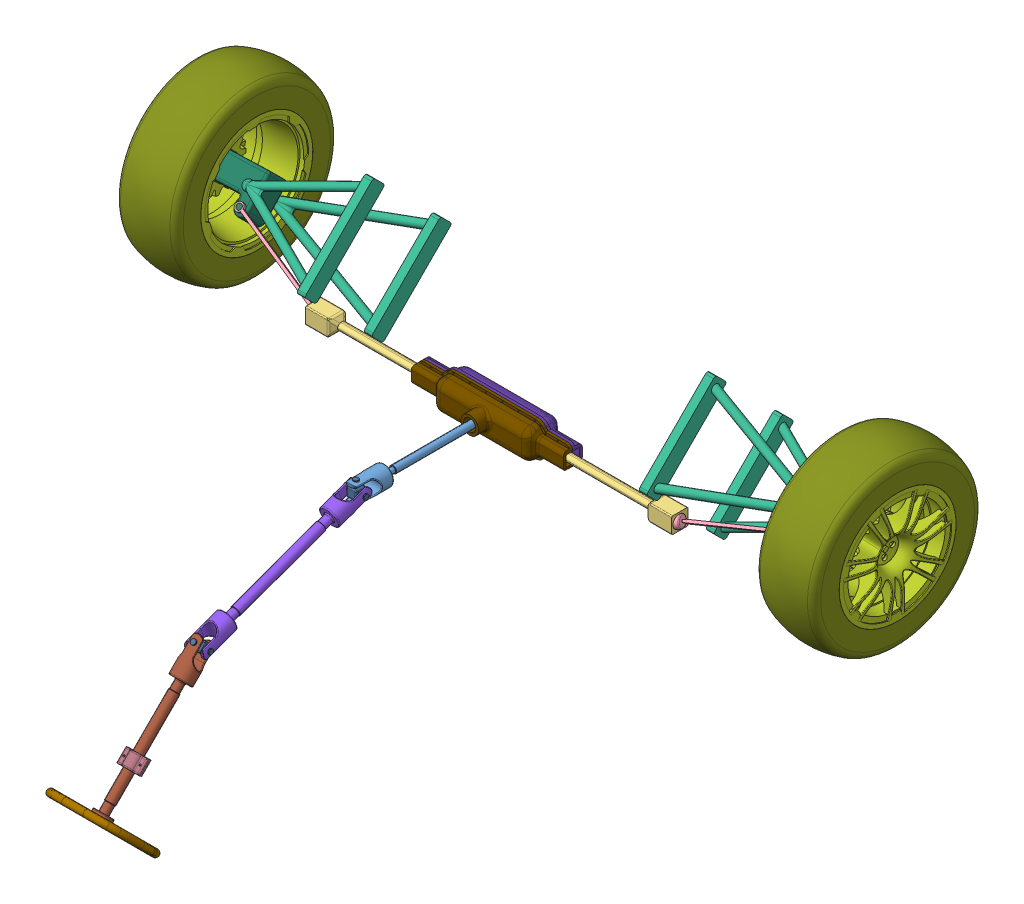
SolidWorks assembly DAS Steering Rack, configuration Default. Lengths in mm.
Overall size (2659.56 1228.41 2209.95).
58 component instances, 18 part files, 66 mates.
Components (placement in the parent):
- Gear Shaft & Helical Gears-1: Gear Shaft & Helical Gears [Default] at (0 0 15) x (1 -0.000577 0) z (0 0 1) size (72 72 565)
- Outer Gear-3: Outer Gear [Front] x (-1 0.000577 0) z (0 0 1) size (11.91 11.4 20)
- Outer Gear-4: Outer Gear [Rear] at (0 0 20) x (-0.809356 -0.587318 0) z (0 0 1) size (11.91 11.4 20)
- Rack-1: Rack [Default] at (-0.0029 -44.7422 0) size (815 60 60.74)
- Rack-2: Rack [Default] at (-0.0029 -44.7422 0) x (-1 0 0) z (0 0 -1) size (815 60 60.74)
- Tie rod-5: Tie rod [Default] at (667.4951 -20.1559 0) x (-0.342021 0.664463 -0.664463) z (0.939692 0.241845 -0.241845) size (48 48 439)
- Steering Arm (Right)-2: Steering Arm (Right) [Default] at (1035.4478 87.5754 -185.513) x (-0.035044 -0.706672 0.706672) z (-0.999386 0.02478 -0.02478) size (146.94 110 180)
- Wheel Tether-3: Wheel Tether [Default] at (645.4747 126.0537 -132.0674) x (-1 0 0) z (0 0.707107 -0.707107) size (447.5 180 360)
- Rim for DAS replica-1: Rim for DAS replica [Default] at (1284.1967 85.5753 -183.5129) x (0.999386 -0.02478 0.02478) z (-0.02478 0.000307 0.999693) size (247.04 420 420)
- Steering Shaft-1: Steering Shaft [Double Yoke] at (0 -104.1602 805.7221) x (0.000614 0.939692 0.34202) z (0 -0.34202 0.939693) size (72 72 660)
- Steering Wheel-1: Steering Wheel [Default] at (0 -580.6434 1464.2229) x (-1 0.000393 0.000393) z (0 0.707107 -0.707107) size (325.52 275 26.89)
- UJ Cross-1: UJ Cross [Default] at (0 0 519.5442) x (-0.000577 -1 0) z (1 -0.000577 -0.00021) size (78 36 78)
- Shaft with wheel hub-1: Shaft with wheel hub [Default] at (0 -579.2292 1462.8087) x (1 -0.000393 -0.000393) z (0 0.707107 -0.707107) size (72 72 550)
- UJ Cross-2: UJ Cross [Default] at (0 -208.3205 1091.8999) x (1 -0.000577 -0.00021) z (0.000556 0.707107 0.707107) size (78 36 78)
- cross countersunk head screw_as-1: cross countersunk head screw_as [AS-NZS 1023 CC- M4 x 16-N] at (0.0139 -564.582 1483.5168) x (0 0.707107 -0.707107) z (0.707107 0.5 0.5) size (16 8.4 8.4)
- Gear Shaft guide-2: Gear Shaft guide [Bottom of Screw Hole] at (0 -436.2108 1319.7902) x (1 0 0) z (0 -0.707107 0.707107) size (81.42 23 50)
- Gear Shaft guide-3: Gear Shaft guide [Top of Screw Hole] at (0 -472.1283 1355.7078) x (-1 0 0) z (0 0.707107 -0.707107) size (81.42 23 50)
- cross countersunk head screw_as-2: cross countersunk head screw_as [AS-NZS 1023 CC- M4 x 16-N] at (-21.6437 -573.4124 1474.6865) x (0 0.707107 -0.707107) z (0.707107 0.5 0.5) size (16 8.4 8.4)
- cross countersunk head screw_as-3: cross countersunk head screw_as [AS-NZS 1023 CC- M4 x 16-N] at (21.6576 -573.4294 1474.6695) x (0 0.707107 -0.707107) z (0.707107 0.5 0.5) size (16 8.4 8.4)
- cross countersunk head screw_as-4: cross countersunk head screw_as [AS-NZS 1023 CC- M4 x 16-N] at (-21.6576 -591.09 1457.0089) x (0 0.707107 -0.707107) z (-0.70632 0.500556 0.500556) size (16 8.4 8.4)
- cross countersunk head screw_as-5: cross countersunk head screw_as [AS-NZS 1023 CC- M4 x 16-N] at (-0.0139 -599.9374 1448.1615) x (0 0.707107 -0.707107) z (-0.70632 0.500556 0.500556) size (16 8.4 8.4)
- cross countersunk head screw_as-6: cross countersunk head screw_as [AS-NZS 1023 CC- M4 x 16-N] at (21.6437 -591.1071 1456.9918) x (0 0.707107 -0.707107) z (-0.70632 0.500556 0.500556) size (16 8.4 8.4)
- flat head screw_am-1: flat head screw_am [B18.6.7M - M3 x 0.5 x 20 Type I Cross Recessed FHMS --20N] at (-29.5627 -447.0631 1344.8554) x (0 -0.707107 -0.707107) z (0.707107 -0.5 0.5) size (20 5.5 5.5)
- flat head screw_am-2: flat head screw_am [B18.6.7M - M3 x 0.5 x 20 Type I Cross Recessed FHMS --20N] at (29.5627 -447.0631 1344.8554) x (0 -0.707107 -0.707107) z (0.707107 -0.5 0.5) size (20 5.5 5.5)
- Rim for DAS replica-3: Rim for DAS replica [Default] at (-1283.5284 87.2394 -185.1771) x (-0.999681 -0.017858 0.017858) z (-0.020657 0.984994 -0.171347) size (247.04 420 420)
- Steering Arm (Left)-1: Steering Arm (Left) [Default] at (-1034.7637 87.5169 -185.4546) x (0.025256 -0.706881 0.706881) z (-0.999681 -0.017858 0.017858) size (146.94 110 180)
- Tie rod-8: Tie rod [Default] at (-667.5009 -20.1559 0) x (-0.342017 -0.664464 0.664464) z (-0.939694 0.241842 -0.241842) size (48 48 439)
- Wheel Tether-5: Wheel Tether [Default] at (-644.8938 126.065 -132.0787) x (1 0 0) z (0 -0.707107 0.707107) size (447.5 180 360)
- Tyre-1: Tyre [Default] at (-1283.5284 87.2394 -185.1771) x (-0.999681 -0.017858 0.017858) z (-0.006607 0.867402 0.497563) size (220 638.99 638.99)
- Tyre-2: Tyre [Default] at (1284.1967 85.5753 -183.5129) x (0.999386 -0.02478 0.02478) z (-0.034928 -0.646862 0.761807) size (220 638.99 638.99)
- Front Shell-1: Front Shell [Default] at (0 -12.05 0) size (560 126.32 60)
- Rear Shell-1: Rear Shell [Default] at (0 -12.05 0) size (560 126.32 100)
- Wheel Tether-6: Wheel Tether [Default] at (645.4747 34.1298 -223.9913) x (-1 0 0) z (0 -0.707107 0.707107) size (447.5 180 360)
- Wheel Tether-7: Wheel Tether [Default] at (-645.4747 34.1298 -223.9913) x (1 0 0) z (0 0.707107 -0.707107) size (447.5 180 360)
- cross countersunk head screw_as-19: cross countersunk head screw_as [AS-NZS 1023 CC- M2 x 20-N] at (-233.7016 23.0571 10.2343) x (0 0 -1) z (1 0 0) size (20 3.8 3.8)
- cross countersunk head screw_as-20: cross countersunk head screw_as [AS-NZS 1023 CC- M2 x 20-N] at (189.2362 23.0571 10.2343) x (0 0 -1) z (1 0 0) size (20 3.8 3.8)
- cross countersunk head screw_as-21: cross countersunk head screw_as [AS-NZS 1023 CC- M2 x 20-N] at (-149.8105 46.1 10.2343) x (0 0 -1) z (1 0 0) size (20 3.8 3.8)
- cross countersunk head screw_as-22: cross countersunk head screw_as [AS-NZS 1023 CC- M2 x 20-N] at (30.1895 46.1 10.2343) x (0 0 -1) z (1 0 0) size (20 3.8 3.8)
- cross countersunk head screw_as-23: cross countersunk head screw_as [AS-NZS 1023 CC- M2 x 20-N] at (-189.2362 23.0571 10.2343) x (0 0 -1) z (1 0 0) size (20 3.8 3.8)
- cross countersunk head screw_as-24: cross countersunk head screw_as [AS-NZS 1023 CC- M2 x 20-N] at (-29.8105 46.1 10.2343) x (0 0 -1) z (1 0 0) size (20 3.8 3.8)
- cross countersunk head screw_as-25: cross countersunk head screw_as [AS-NZS 1023 CC- M2 x 20-N] at (233.7016 23.0571 10.2343) x (0 0 -1) z (1 0 0) size (20 3.8 3.8)
- cross countersunk head screw_as-26: cross countersunk head screw_as [AS-NZS 1023 CC- M2 x 20-N] at (171.1012 39.2432 10.2343) x (0 0 -1) z (1 0 0) size (20 3.8 3.8)
- cross countersunk head screw_as-27: cross countersunk head screw_as [AS-NZS 1023 CC- M2 x 20-N] at (-89.8105 46.1 10.2343) x (0 0 -1) z (1 0 0) size (20 3.8 3.8)
- cross countersunk head screw_as-28: cross countersunk head screw_as [AS-NZS 1023 CC- M2 x 20-N] at (90.1895 46.1 10.2343) x (0 0 -1) z (1 0 0) size (20 3.8 3.8)
- cross countersunk head screw_as-29: cross countersunk head screw_as [AS-NZS 1023 CC- M2 x 20-N] at (149.8685 46.1 10.2343) x (0 0 -1) z (1 0 0) size (20 3.8 3.8)
- cross countersunk head screw_as-30: cross countersunk head screw_as [AS-NZS 1023 CC- M2 x 20-N] at (-171.1012 39.2432 10.2343) x (0 0 -1) z (1 0 0) size (20 3.8 3.8)
- cross countersunk head screw_as-31: cross countersunk head screw_as [AS-NZS 1023 CC- M2 x 20-N] at (-233.7016 -47.1571 10.2343) x (0 0 -1) z (-1 0 0) size (20 3.8 3.8)
- cross countersunk head screw_as-32: cross countersunk head screw_as [AS-NZS 1023 CC- M2 x 20-N] at (189.2362 -47.1571 10.2343) x (0 0 -1) z (-1 0 0) size (20 3.8 3.8)
- cross countersunk head screw_as-33: cross countersunk head screw_as [AS-NZS 1023 CC- M2 x 20-N] at (-149.8105 -70.2 10.2343) x (0 0 -1) z (-1 0 0) size (20 3.8 3.8)
- cross countersunk head screw_as-34: cross countersunk head screw_as [AS-NZS 1023 CC- M2 x 20-N] at (30.1895 -70.2 10.2343) x (0 0 -1) z (-1 0 0) size (20 3.8 3.8)
- cross countersunk head screw_as-35: cross countersunk head screw_as [AS-NZS 1023 CC- M2 x 20-N] at (-189.2362 -47.1571 10.2343) x (0 0 -1) z (-1 0 0) size (20 3.8 3.8)
- cross countersunk head screw_as-36: cross countersunk head screw_as [AS-NZS 1023 CC- M2 x 20-N] at (-29.8105 -70.2 10.2343) x (0 0 -1) z (-1 0 0) size (20 3.8 3.8)
- cross countersunk head screw_as-37: cross countersunk head screw_as [AS-NZS 1023 CC- M2 x 20-N] at (233.7016 -47.1571 10.2343) x (0 0 -1) z (-1 0 0) size (20 3.8 3.8)
- cross countersunk head screw_as-38: cross countersunk head screw_as [AS-NZS 1023 CC- M2 x 20-N] at (171.1012 -63.3432 10.2343) x (0 0 -1) z (-1 0 0) size (20 3.8 3.8)
- cross countersunk head screw_as-39: cross countersunk head screw_as [AS-NZS 1023 CC- M2 x 20-N] at (-89.8105 -70.2 10.2343) x (0 0 -1) z (-1 0 0) size (20 3.8 3.8)
- cross countersunk head screw_as-40: cross countersunk head screw_as [AS-NZS 1023 CC- M2 x 20-N] at (90.1895 -70.2 10.2343) x (0 0 -1) z (-1 0 0) size (20 3.8 3.8)
- cross countersunk head screw_as-41: cross countersunk head screw_as [AS-NZS 1023 CC- M2 x 20-N] at (149.8685 -70.2 10.2343) x (0 0 -1) z (-1 0 0) size (20 3.8 3.8)
- cross countersunk head screw_as-42: cross countersunk head screw_as [AS-NZS 1023 CC- M2 x 20-N] at (-171.1012 -63.3432 10.2343) x (0 0 -1) z (-1 0 0) size (20 3.8 3.8)
Mates (geometry in assembly coordinates):
- Coincident1: coincident aligned: line of Gear Shaft & Helical Gears-1 through (0 0 48.1432) axis (0 0 1)
- Coincident2: coincident aligned: line of Gear Shaft & Helical Gears-1 through (0 0 48.1432) axis (0 0 1)
- Coincident3: coincident anti-aligned: line of Gear Shaft & Helical Gears-1 through (0 0 -20) axis (0 0 1); line of Outer Gear-3 through (0 0 0) axis (0 0 -1)
- PathMate1: path: point of Outer Gear-3; curve of Gear Shaft & Helical Gears-1
- Distance1: distance = 20 mm anti-aligned: plane of Outer Gear-3 through (2.2501 0.6145 -20) normal (0 0 -1)
- Coincident4: coincident anti-aligned: plane of Outer Gear-4 through (1.4592 1.8197 0) normal (0 0 -1)
- PathMate2: path: point of Outer Gear-4; curve of Gear Shaft & Helical Gears-1
- Coincident5: coincident anti-aligned: line of Gear Shaft & Helical Gears-1 through (0 0 48.1432) axis (0 0 1); line of Outer Gear-4 through (0 0 20) axis (0 0 -1)
- Coincident6: coincident anti-aligned: plane of Rack-2 through (1.5679 -44.7422 0) normal (0 0 -1)
- RackPinionMate1: rack pinion = 10 mm: line of Rack-2 through (-142.5009 -30.2 0) axis (1 0 0); cylinder of Outer Gear-4 through (0 0 20) axis (0 0 -1) radius 5.9572
- Coincident7: coincident aligned: plane of assembly through (0 0 0) normal (0 0 1); plane of Rack-1 through (-1.5737 -44.7422 0) normal (0 0 1)
- RackPinionMate2: rack pinion = 10 mm: line of Rack-1 through (142.4951 -30.2 -25) axis (-1 0 0); cylinder of Outer Gear-3 through (0 0 0) axis (0 0 -1) radius 5.9572
- LimitDistance1: limit distance = 0 mm anti-aligned: plane of Gear Shaft & Helical Gears-1 through (0 0 25) normal (0 0 -1); plane of Rack-2 through (-0.0029 -44.7422 25) normal (0 0 1)
- Concentric1: concentric: sphere of Rack-2; sphere of Tie rod-5
- Parallel1: parallel anti-aligned: plane of Tie rod-5 through (1045.0822 76.7955 -89.8803) normal (0 0.707107 0.707107)
- Concentric2: concentric anti-aligned: cylinder of Tie rod-5 through (1043.3721 53.0467 -120.2737) axis (0 0.707107 0.707107) radius 10; cylinder of Steering Arm (Right)-2 through (1043.3721 80.1178 -93.2026) axis (0 -0.707107 -0.707107) radius 10
- Coincident8: coincident aligned: plane of Tie rod-5 through (1045.0822 76.7955 -89.8803) normal (0 0.707107 0.707107); plane of Steering Arm (Right)-2 through (1043.3721 80.1178 -93.2026) normal (0 0.707107 0.707107)
- Concentric3: concentric aligned: cylinder of Steering Arm (Right)-2 through (1045.4747 97.7694 -160.3517) axis (0 0.707107 0.707107) radius 17.5; cylinder of Wheel Tether-3 through (1045.4747 97.7694 -160.3517) axis (0 0.707107 0.707107) radius 17.5
- Coincident9: coincident anti-aligned: plane of Steering Arm (Right)-2 through (1200.9443 87.6396 -185.5772) normal (0.999386 -0.02478 0.02478); plane of Rim for DAS replica-1 through (1202.0551 132.4541 -185.5634) normal (-0.999386 0.02478 -0.02478)
- Concentric4: concentric aligned: cylinder of Steering Arm (Right)-2 through (1200.9443 87.6396 -185.5772) axis (-0.999386 0.02478 -0.02478) radius 45.8283; cylinder of Rim for DAS replica-1 through (1202.6242 87.5979 -185.5355) axis (-0.999386 0.02478 -0.02478) radius 42.8283
- Coincident10: coincident: line of Gear Shaft & Helical Gears-1 through (0 0 535.4731) axis (0 0 -1); unknown of UJ Cross-1
- Concentric5: concentric anti-aligned: cylinder of Gear Shaft & Helical Gears-1 through (-0.0208 -36 519.5442) axis (0.000577 1 0) radius 7.5; cylinder of UJ Cross-1 through (0.0219 38 519.5442) axis (-0.000577 -1 0) radius 7
- Coincident11: coincident: line of Steering Shaft-1 through (0 5.448 504.5759) axis (0 -0.34202 0.939693); unknown of UJ Cross-1
- Concentric6: concentric anti-aligned: circle of Steering Shaft-1; cylinder of UJ Cross-1 through (-38 0.0219 519.5521) axis (1 -0.000577 -0.00021) radius 7
- Coincident12: coincident: line of Steering Shaft-1 through (0 -47.0913 648.9265) axis (0 -0.34202 0.939693)
- Coincident13: coincident: line of Steering Shaft-1 through (0 -213.7685 1106.8682) axis (0 0.34202 -0.939693); unknown of UJ Cross-2
- Concentric7: concentric aligned: cylinder of Steering Shaft-1 through (36 -208.3412 1091.8924) axis (-1 0.000577 0.00021) radius 7.5; cylinder of UJ Cross-2 through (38 -208.3424 1091.892) axis (-1 0.000577 0.00021) radius 7
- Coincident14: coincident: line of Shaft with wheel hub-1 through (0 -197.057 1080.6365) axis (0 -0.707107 0.707107); unknown of UJ Cross-2
- Concentric8: concentric aligned: cylinder of Shaft with wheel hub-1 through (0.02 -182.8646 1117.3558) axis (-0.000556 -0.707107 -0.707107) radius 7.5; cylinder of UJ Cross-2 through (0.0211 -181.4504 1118.77) axis (-0.000556 -0.707107 -0.707107) radius 7
- Coincident15: coincident: line of Shaft with wheel hub-1 through (0 -541.6523 1425.2318) axis (0 0.707107 -0.707107)
- Concentric9: concentric aligned: cylinder of Steering Wheel-1 through (21.6576 -573.2273 1474.4674) axis (0 -0.707107 0.707107) radius 2.15; cylinder of Shaft with wheel hub-1 through (21.6576 -566.8634 1468.1035) axis (0 -0.707107 0.707107) radius 2.15
- Concentric10: concentric aligned: cylinder of Steering Wheel-1 through (-21.6576 -590.8879 1456.8068) axis (0 -0.707107 0.707107) radius 2.15; cylinder of Shaft with wheel hub-1 through (-21.6576 -584.524 1450.4428) axis (0 -0.707107 0.707107) radius 2.15
- Coincident16: coincident anti-aligned: plane of Steering Wheel-1 through (80.9346 -616.6111 1425.4268) normal (0 0.707107 -0.707107); plane of Shaft with wheel hub-1 through (0 -579.2292 1462.8087) normal (0 -0.707107 0.707107)
- Coincident17: coincident aligned: cone of Steering Wheel-1 through (0.0139 -564.38 1483.3148) axis (0 0.707107 -0.707107); cone of cross countersunk head screw_as-1 through (0.0139 -562.6728 1481.6077) axis (0 0.707107 -0.707107)
- Concentric11: concentric aligned: cylinder of Shaft with wheel hub-1 through (0 -282.2444 1165.8238) axis (0 0.707107 -0.707107) radius 17; cylinder of Gear Shaft guide-2 through (0 -471.5661 1355.1456) axis (0 0.707107 -0.707107) radius 13
- Coincident18: coincident aligned: cone of Steering Wheel-1 through (-21.6437 -573.2103 1474.4845) axis (0 0.707107 -0.707107); cone of cross countersunk head screw_as-2 through (-21.6437 -571.5032 1472.7773) axis (0 0.707107 -0.707107)
- Coincident19: coincident aligned: cone of Steering Wheel-1 through (21.6576 -573.2273 1474.4674) axis (0 0.707107 -0.707107); cone of cross countersunk head screw_as-3 through (21.6576 -571.5202 1472.7603) axis (0 0.707107 -0.707107)
- Coincident20: coincident aligned: cone of Gear Shaft guide-3 through (-29.5627 -447.0985 1344.8201) axis (0 -0.707107 -0.707107); cone of flat head screw_am-1 through (-29.5627 -447.3813 1344.5372) axis (0 -0.707107 -0.707107)
- Coincident21: coincident aligned: cone of Gear Shaft guide-3 through (29.5627 -447.0985 1344.8201) axis (0 -0.707107 -0.707107); cone of flat head screw_am-2 through (29.5627 -447.3813 1344.5372) axis (0 -0.707107 -0.707107)
- Concentric12: concentric: sphere of Rack-1; sphere of Tie rod-8
- Parallel28: parallel anti-aligned: plane of Tie rod-8 through (-1041.6684 83.4389 -96.5237) normal (0 0.707107 0.707107)
- Coincident22: coincident aligned: plane of Steering Arm (Left)-1 through (-1043.3785 80.1166 -93.2014) normal (0 0.707107 0.707107); plane of Tie rod-8 through (-1041.6684 83.4389 -96.5237) normal (0 0.707107 0.707107)
- Concentric13: concentric anti-aligned: cylinder of Steering Arm (Left)-1 through (-1043.3785 80.1166 -93.2014) axis (0 -0.707107 -0.707107) radius 10; cylinder of Tie rod-8 through (-1043.3785 53.0455 -120.2724) axis (0 0.707107 0.707107) radius 10
- Concentric14: concentric aligned: cylinder of Steering Arm (Left)-1 through (-1044.8938 97.7807 -160.363) axis (0 0.707107 0.707107) radius 17.5; cylinder of Wheel Tether-5 through (-1044.8938 97.7807 -160.363) axis (0 0.707107 0.707107) radius 17.5
- Concentric15: concentric aligned: cylinder of Rim for DAS replica-3 through (-1201.9318 88.6971 -186.6347) axis (0.999681 0.017858 -0.017858) radius 42.8283; cylinder of Steering Arm (Left)-1 through (-1195.253 88.8164 -186.754) axis (0.999681 0.017858 -0.017858) radius 42.8283
- Coincident23: coincident anti-aligned: plane of Rim for DAS replica-3 through (-1199.6 96.4224 -142.5066) normal (0.999681 0.017858 -0.017858); plane of Steering Arm (Left)-1 through (-1200.2514 88.7271 -186.6647) normal (-0.999681 -0.017858 0.017858)
- Coincident24: coincident anti-aligned: plane of Rack-1 through (142.4951 -30.2 -20) normal (0 -1 0)
- Coincident25: coincident anti-aligned: plane of Rack-2 through (-142.5009 -30.2 20) normal (0 -1 0)
- Concentric16: concentric aligned: cylinder of Rim for DAS replica-3 through (-1283.5284 87.2394 -185.1771) axis (-0.999681 -0.017858 0.017858) radius 210; cylinder of Tyre-1 through (-1283.5284 87.2394 -185.1771) axis (-0.999681 -0.017858 0.017858) radius 210.4
- Coincident26: coincident aligned: plane of Rim for DAS replica-3 through (-1073.5954 90.9897 -188.9273) normal (0.999681 0.017858 -0.017858); plane of Tyre-1 through (-1073.5954 90.9897 -188.9273) normal (0.999681 0.017858 -0.017858)
- Concentric17: concentric aligned: cylinder of Rim for DAS replica-1 through (1284.1967 85.5753 -183.5129) axis (0.999386 -0.02478 0.02478) radius 210; cylinder of Tyre-2 through (1284.1967 85.5753 -183.5129) axis (0.999386 -0.02478 0.02478) radius 210.4
- Coincident28: coincident aligned: plane of Rim for DAS replica-1 through (1074.3257 90.7791 -188.7167) normal (-0.999386 0.02478 -0.02478); plane of Tyre-2 through (1074.3257 90.7791 -188.7167) normal (-0.999386 0.02478 -0.02478)
- Coincident29: coincident aligned: cone of Rear Shell-1 through (-233.7016 23.0571 10) axis (0 0 -1); cone of cross countersunk head screw_as-19 through (-233.7016 23.0571 9.0343) axis (0 0 -1)
- Coincident30: coincident aligned: cone of Rear Shell-1 through (-189.2362 23.0571 10) axis (0 0 -1); cone of cross countersunk head screw_as-23 through (-189.2362 23.0571 9.0343) axis (0 0 -1)
- Coincident31: coincident aligned: cone of Rear Shell-1 through (-89.8105 46.1 10) axis (0 0 -1); cone of cross countersunk head screw_as-27 through (-89.8105 46.1 9.0343) axis (0 0 -1)
- Coincident32: coincident aligned: cone of Rear Shell-1 through (-29.8105 46.1 10) axis (0 0 -1); cone of cross countersunk head screw_as-24 through (-29.8105 46.1 9.0343) axis (0 0 -1)
- Coincident33: coincident aligned: cone of Rear Shell-1 through (30.1895 46.1 10) axis (0 0 -1); cone of cross countersunk head screw_as-22 through (30.1895 46.1 9.0343) axis (0 0 -1)
- Coincident34: coincident aligned: cone of Rear Shell-1 through (90.1895 46.1 10) axis (0 0 -1); cone of cross countersunk head screw_as-28 through (90.1895 46.1 9.0343) axis (0 0 -1)
- Coincident35: coincident aligned: cone of Rear Shell-1 through (149.8685 46.1 10) axis (0 0 -1); cone of cross countersunk head screw_as-29 through (149.8685 46.1 9.0343) axis (0 0 -1)
- Coincident36: coincident aligned: cone of Rear Shell-1 through (171.1012 39.2432 10) axis (0 0 -1); cone of cross countersunk head screw_as-26 through (171.1012 39.2432 9.0343) axis (0 0 -1)
- Coincident37: coincident aligned: cone of Rear Shell-1 through (189.2362 23.0571 10) axis (0 0 -1); cone of cross countersunk head screw_as-20 through (189.2362 23.0571 9.0343) axis (0 0 -1)
- Coincident38: coincident aligned: cone of Rear Shell-1 through (233.7016 23.0571 10) axis (0 0 -1); cone of cross countersunk head screw_as-25 through (233.7016 23.0571 9.0343) axis (0 0 -1)
- Coincident39: coincident aligned: cone of Rear Shell-1 through (-149.8105 46.1 10) axis (0 0 -1); cone of cross countersunk head screw_as-21 through (-149.8105 46.1 9.0343) axis (0 0 -1)
- Coincident40: coincident aligned: cone of Rear Shell-1 through (-171.1012 39.2432 10) axis (0 0 -1); cone of cross countersunk head screw_as-30 through (-171.1012 39.2432 9.0343) axis (0 0 -1)
- Parallel31: parallel: plane of assembly through (0 -13.1221 -13.1221) normal (0 -0.707107 -0.707107); plane of Steering Wheel-1; plane of assembly
- Parallel36: parallel: plane of assembly through (0 -13.1221 -13.1221) normal (0 -0.707107 -0.707107); plane of Steering Wheel-1 through (0 -580.709 1464.2885) normal (-0.068226 0.705459 0.705459); plane of assembly
